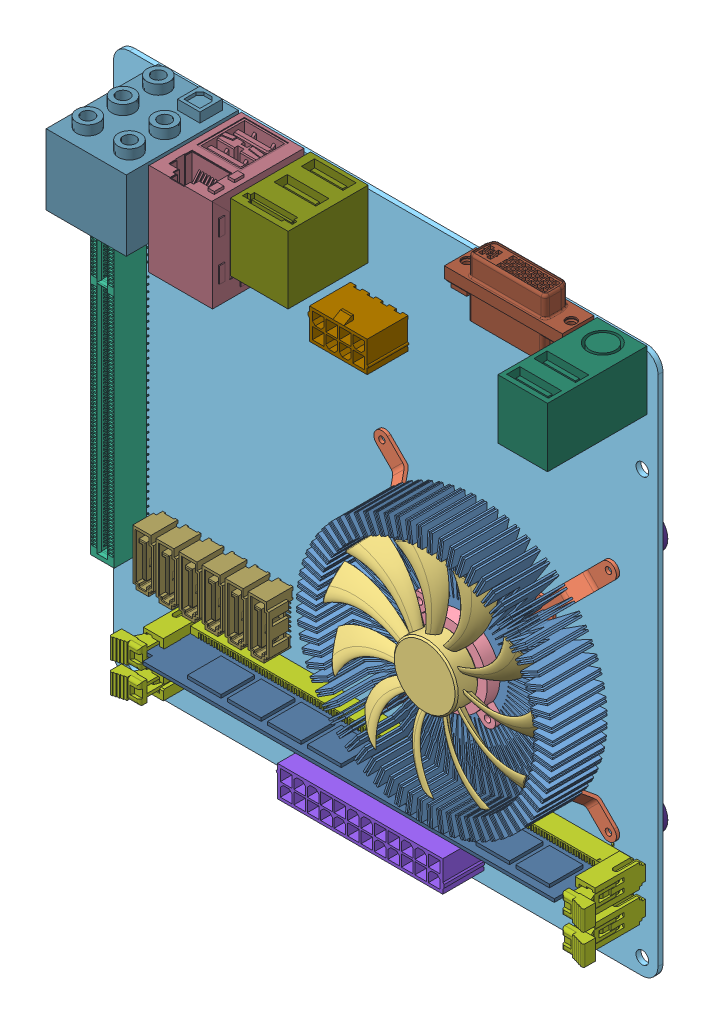
SolidWorks assembly Assem1, configuration Predeterminado. Lengths in mm.
Overall size (199.39 177.44 41.55).
26 component instances, 18 part files, 0 mates.
Components (placement in the parent):
- asrock-z87e-itx.stp-1: asrock-z87e-itx.stp [Predeterminado] at (3.9521 -38.631 183.6159) size (199.39 177.44 41.55)
  - cooling-fan-silverstone-nt07-115x.stp-1: cooling-fan-silverstone-nt07-115x.stp [Predeterminado] at (40.1446 -10.0696 12.55) x (0.707107 0.707107 0) z (0.707107 -0.707107 0) size (105 23 105)
    - 01.stp-1: 01.stp [Predeterminado] at origin size (79.98 17 79.98)
    - 02.stp-1: 02.stp [Predeterminado] at (0 0 0) x (-1 0 0) z (0 -1 0) size (105 105 6)
    - 03.stp-1: 03.stp [Predeterminado] at (0 10 0) x (0.309828 0 0.950793) z (-0.950793 0 0.309828) size (66.74 7 66.79)
    - 04.stp-1: 04.stp [Predeterminado] at (0 6 0) size (25 4 35)
  - mini-ITX-substrate.stp-1: mini-ITX-substrate.stp [Predeterminado] at origin size (170 170 1.55)
  - pcie-socket.stp-1: pcie-socket.stp [Predeterminado] at (-92.83 -11.23 2.69) x (0 -1 0) z (0 0 1) size (89 8.85 15.63)
  - ddr3-socket.stp-1: ddr3-socket.stp [Predeterminado] at (-60 -69.775 8.72) x (-1 0 0) z (0 1 0) size (148 26.69 7.35)
  - ddr3-socket.stp-2: ddr3-socket.stp [Predeterminado] at (-60 -60.275 8.72) x (-1 0 0) z (0 1 0) size (148 26.69 7.35)
  - atx-24-circuits-molex.stp-1: atx-24-circuits-molex.stp [Predeterminado] at (4.8 -76.45 1.55) x (-1 0 0) z (0 1 0) size (52.4 16.3 11)
  - atx-8-circuits-molex.stp-1: atx-8-circuits-molex.stp [Predeterminado] at (-2 52.2 1.55) x (1 0 0) z (0 -1 0) size (18.8 16.3 11)
  - ddr3-4Gbyte-ram-module-kingston.stp-1: ddr3-4Gbyte-ram-module-kingston.stp [Predeterminado] at (10.4 -56.875 14.05) x (1 0 0) z (0 1 0) size (133 19 2)
  - dvi-connector.stp-1: dvi-connector.stp [Predeterminado] at (46.6 86 6.5) x (-1 0 0) z (0 1 0) size (36.8 12.4 17.94)
  - sata-header-molex.stp-1: sata-header-molex.stp [Predeterminado] at (-67.325 -42.65 5.75) x (0 -1 0) z (0 0 1) size (16.9 6.45 11.05)
  - sata-header-molex.stp-2: sata-header-molex.stp [Predeterminado] at (-60.125 -42.65 5.75) x (0 -1 0) z (0 0 1) size (16.9 6.45 11.05)
  - sata-header-molex.stp-3: sata-header-molex.stp [Predeterminado] at (-52.925 -42.65 5.75) x (0 -1 0) z (0 0 1) size (16.9 6.45 11.05)
  - sata-header-molex.stp-4: sata-header-molex.stp [Predeterminado] at (-45.725 -42.65 5.75) x (0 -1 0) z (0 0 1) size (16.9 6.45 11.05)
  - sata-header-molex.stp-5: sata-header-molex.stp [Predeterminado] at (-38.525 -42.65 5.75) x (0 -1 0) z (0 0 1) size (16.9 6.45 11.05)
  - sata-header-molex.stp-6: sata-header-molex.stp [Predeterminado] at (-31.325 -42.65 5.75) x (0 -1 0) z (0 0 1) size (16.9 6.45 11.05)
  - hdmi-receptacle-dual.stp-1: hdmi-receptacle-dual.stp [Predeterminado] at (17.15 86 10.825) x (-1 0 0) z (0 1 0)
  - rj45-dual-usb-combo.stp-1: rj45-dual-usb-combo.stp [Predeterminado] at (-35.245 86 15.965) x (-1 0 0) z (0 1 0) size (20.71 33 29.77)
  - audio-jacks-receptacle.stp-1: audio-jacks-receptacle.stp [Predeterminado] at (-58.5 75 1.55) x (-1 0 0) z (0 0 1) size (25 25 35)
  - ps2-dual-usb-receptacle.stp-1: ps2-dual-usb-receptacle.stp [Predeterminado] at (73.75 76.75 1.55) x (-1 0 0) z (0 0 1) size (15.5 18.5 31)
  - esata-dual-usb-receptacle.stp-1: esata-dual-usb-receptacle.stp [Predeterminado] at (-14.49 75.5 1.55) x (-1 0 0) z (0 0 1) size (18 21 25)
  - fan-holding-base.stp-1: fan-holding-base.stp [Predeterminado] at (37.4999 -7.4249 -5) size (88 88 5)
